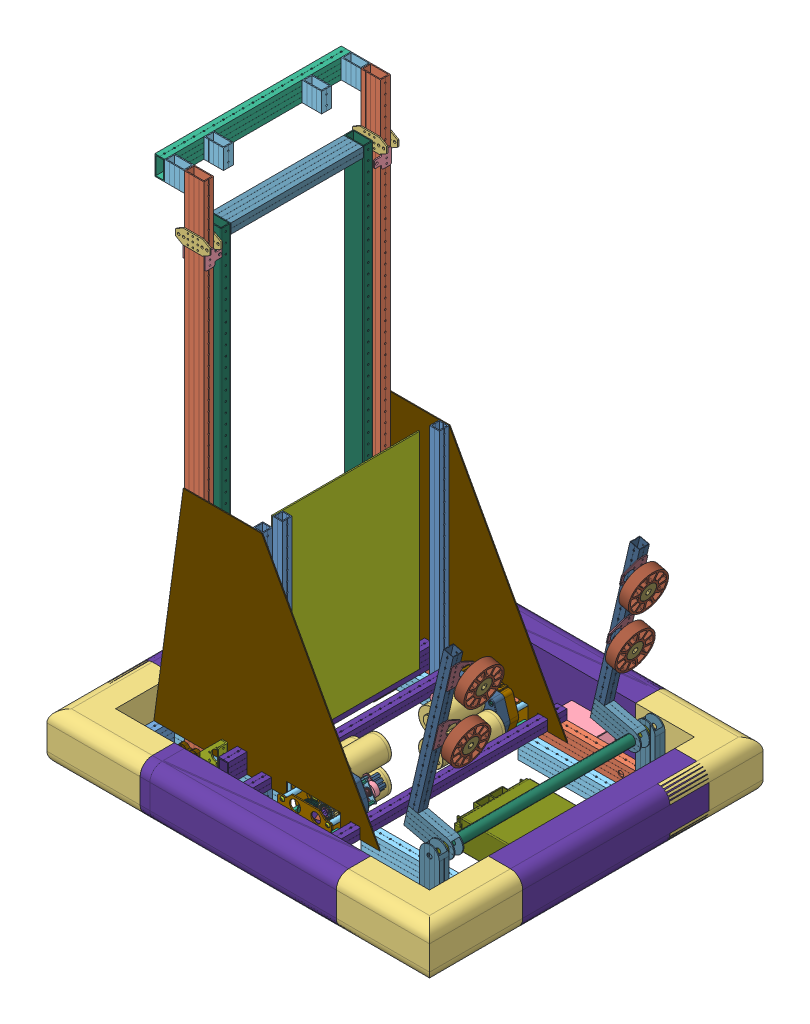
SolidWorks assembly FINAL BOT, configuration Default. Lengths in mm. (continued)
Components (placement in the parent): (continued)
- Elevator Moving Stage-2: Elevator Moving Stage [Default] at (1084.9152 646.5878 79.8495) x (0 0 1) z (-1 0 0) size (444.5 1143 88.9)
  - Elevator Crossbar-1: Elevator Crossbar [Default] at (70.321 -334.7906 927.1918) x (0 1 0) z (1 0 0) size (25.4 50.8 342.9)
  - Elevator Crossbar-2: Elevator Crossbar [Default] at (70.321 738.3594 927.1918) x (0 1 0) z (1 0 0) size (25.4 50.8 342.9)
  - Linear Motion Gusset-2: Linear Motion Gusset [Default] at (479.8486 -372.4027 926.9137) x (0 0 1) z (-1 0 0) size (88.9 73.03 47.09)
    - 217-4399-001 Rev2-1: 217-4399-001 Rev2 [Default] at (0.2781 -0.4879 -0.0474) size (88.9 38.1 3.17)
    - 217-4399-001 Rev2-2: 217-4399-001 Rev2 [Default] at (0.2781 -0.4879 28.5276) size (88.9 38.1 3.17)
    - 217-4399-005 Rev2-1: 217-4399-005 Rev2 [Default] at (25.6781 32.8496 44.0216) x (0 1 0) z (1 0 0) size (41.28 43.91 3.18)
    - 217-4399-005 Rev2-2: 217-4399-005 Rev2 [Default] at (-28.2969 32.8496 44.0216) x (0 1 0) z (1 0 0) size (41.28 43.91 3.18)
  - Elevator Moving Stage Upright-1: Elevator Moving Stage Upright [Default] at (464.021 1.7594 927.1918) x (1 0 0) z (0 1 0) size (25.4 50.8 1143)
  - Elevator Moving Stage Upright-2: Elevator Moving Stage Upright [Default] at (832.321 1.7594 927.1918) x (1 0 0) z (0 1 0) size (25.4 50.8 1143)
  - Linear Motion Gusset-3: Linear Motion Gusset [Default] at (816.4934 -372.4027 927.47) x (0 0 -1) z (1 0 0) size (88.9 73.03 47.09)
    - 217-4399-001 Rev2-1: 217-4399-001 Rev2 [Default] at (0.2781 -0.4879 -0.0474) size (88.9 38.1 3.17)
    - 217-4399-001 Rev2-2: 217-4399-001 Rev2 [Default] at (0.2781 -0.4879 28.5276) size (88.9 38.1 3.17)
    - 217-4399-005 Rev2-1: 217-4399-005 Rev2 [Default] at (25.6781 32.8496 44.0216) x (0 1 0) z (1 0 0) size (41.28 43.91 3.18)
    - 217-4399-005 Rev2-2: 217-4399-005 Rev2 [Default] at (-28.2969 32.8496 44.0216) x (0 1 0) z (1 0 0) size (41.28 43.91 3.18)
  - Custom Elevator Gusset-1: Custom Elevator Gusset [Default] at (425.921 -390.1537 952.5918) size (101.6 127 3.17)
  - Custom Elevator Gusset-2: Custom Elevator Gusset [Default] at (870.421 -390.1537 955.7668) x (-1 0 0) z (0 0 -1) size (101.6 127 3.17)
- Elevator Drive Assembly-1: Elevator Drive Assembly [Default] at (500.2725 546.5466 390.8173) x (-1 0 0) z (0 0 1) size (95.12 72.01 584.2)
  - Elevator Drive Assembly Base Rail-1: Elevator Drive Assembly Base Rail [Default] at (215.5491 266.4994 -119.9968) size (25.4 50.8 584.2)
  - VersaFrame 2 Inch Wide VersaPlanetary Parallel Mount-1: VersaFrame 2 Inch Wide VersaPlanetary Parallel Mount [Default] at (253.5221 266.4359 258.5902) size (73.53 55.5 69.72)
  - 217-2 Stage Versaplanetary STEP-1: 217-2 Stage Versaplanetary STEP [Default] at (253.5221 266.4359 207.0652) x (-1 0 0) z (0 0 -1) size (44.3 44.3 179.1)
    - 217-2625-001 Rev1-1: 217-2625-001 Rev1 [Default] at origin size (42 42 18)
    - 217-2625-002 Rev1-1: 217-2625-002 Rev1 [Default] at (0 0 -29.4) size (42 42 17.13)
    - 217-2625-003 Rev1-1: 217-2625-003 Rev1 [Default] at (0 0 -43.6478) x (1 0 0) z (0 0 -1) size (17 17 64.12)
    - 217-2625-009 Rev1-1: 217-2625-009 Rev1 [Default] at (0 0 -3.48) x (0 -1 0) z (0 0 -1) size (18 18 13)
    - 217-2816-001 Rev1-1: 217-2816-001 Rev1 [Default] at (0 0 -16.85) x (1 0 0) z (0 0 -1) size (42 42 14.5)
    - 217-2625-007 Rev1_Sun_Driver01-1: 217-2625-007 Rev1_Sun_Driver01 [Default] at (0 0 -11.767) x (0.055822 0.998441 0) z (0 0 1) size (14.49 14.49 12.72)
    - 217-2625-100-1: 217-2625-100 [Default] at (0 0 -18.467) x (0 1 0) z (0 0 1) size (39.26 38.9 12.7)
      - 217-2625-008 Rev1-1: 217-2625-008 Rev1 [Default] at origin size (34.7 34.7 4.7)
      - 217-2625-010 Rev1-1: 217-2625-010 Rev1 [Default] at (0 10.193 3.65) x (0.999813 0.019336 0) z (0 0 1) size (4 4 12)
      - 217-2625-010 Rev1-2: 217-2625-010 Rev1 [Default] at (8.691 -5.3258 3.65) size (4 4 12)
      - 217-2625-010 Rev1-3: 217-2625-010 Rev1 [Default] at (-8.691 -5.3258 3.65) size (4 4 12)
      - 217-2625-005 Rev1_Planet_Revolving_Follower01-1: 217-2625-005 Rev1_Planet_Revolving_Follower01 [Default] at (8.691 -5.3258 6.35) x (0.932816 0.360354 0) z (0 0 1) size (16.91 16.92 8)
      - 217-2625-005 Rev1_Planet_Revolving_Follower01-2: 217-2625-005 Rev1_Planet_Revolving_Follower01 [Default] at (-8.691 -5.3258 6.35) x (-0.932788 -0.360426 0) z (0 0 1) size (16.91 16.92 8)
      - 217-2625-005 Rev1_Planet_Revolving_Follower01-3: 217-2625-005 Rev1_Planet_Revolving_Follower01 [Default] at (0 10.193 6.35) x (0.893583 0.448898 0) z (0 0 1) size (16.91 16.92 8)
    - 217-2822-003 Rev4-1: 217-2822-003 Rev4 [Default] at (0 0 9) x (0 1 0) z (0 0 1) size (42 42 4.8)
    - 217-2625-011 Rev1-1: 217-2625-011 Rev1 [Default] at (0 0 1.37) x (1 0 0) z (0 -1 0) size (8.01 7.5 7.94)
    - SSA_SSA0832-0500ZC-1: SSA_SSA0832-0500ZC [Default] at (17.5 -17.5 10.5) x (0.189399 -0.9819 0) z (-0.9819 -0.189399 0) size (6.73 16.76 6.73)
    - 217-2742-1: 217-2742 [Default] at (0 0 -43.1002) x (0 0 1) z (-1 0 0) size (7 28 28)
    - 217-2742-2: 217-2742 [Default] at (0 0 -51.4002) x (0 0 1) z (-0.997393 0.072165 0) size (7 28 28)
    - SSA_SSA0832-1750ZC-1: SSA_SSA0832-1750ZC [Default] at (17.5 -17.5 -47.261) x (1 0 0) z (0 1 0) size (6.73 48.51 6.73)
    - SSA_SSA0832-1750ZC-2: SSA_SSA0832-1750ZC [Default] at (-17.5 17.5 -47.261) x (1 0 0) z (0 1 0) size (6.73 48.51 6.73)
    - 217-2625-018 Rev1_98541A410-1: 217-2625-018 Rev1_98541A410 [Default] at (0 0 -35.4954) x (0 0 -1) z (0.980859 -0.194721 0) size (1 19.6 17.4)
    - 217-2625-017 Rev1_9714K61-1: 217-2625-017 Rev1_9714K61 [Default] at (0 0 -44.1002) x (-0.695225 0.718792 0) z (-0.718792 -0.695225 0) size (28.51 4.98 30.18)
    - PINL-M020-006-S-1: PINL-M020-006-S [Default] at (-18.5 13.6657 -9.5) x (0 0 -1) z (1 0 0) size (6 2 2)
    - PINL-M020-006-S-2: PINL-M020-006-S [Default] at (-18.5 13.6657 -22.2) x (0 0 -1) z (0.23951 -0.970894 0) size (6 2 2)
    - 217-2816-001 Rev1-2: 217-2816-001 Rev1 [Default] at (0 0 -29.55) x (1 0 0) z (0 0 -1) size (42 42 14.5)
    - 217-3106-000 Rev2_NO SUN-1: 217-3106-000 Rev2_NO SUN [Default] at (0 0 -31.5454) size (40.34 37.58 17.71)
      - 217-3106-002 Rev1_Planet_Revolving_Follower01-1: 217-3106-002 Rev1_Planet_Revolving_Follower01 [Default] at (0 10.2965 6.35) x (0.979503 -0.20143 0) z (0 0 1) size (16.8 16.83 8)
      - 217-3106-003 Rev1-1: 217-3106-003 Rev1 [Default] at origin size (34.7 34.7 4.7)
      - 217-3106-001 Rev1_Sun_Driver01-1: 217-3106-001 Rev1_Sun_Driver01 [Default] at (0 0 9.0125) x (1 0 0) z (0 0 -1) size (14.56 14.56 12.7)
      - 217-3106-002 Rev1_Planet_Revolving_Follower01-2: 217-3106-002 Rev1_Planet_Revolving_Follower01 [Default] at (8.917 -5.1482 6.35) x (-0.664195 -0.74756 0) z (0 0 1) size (16.8 16.83 8)
      - 217-3106-002 Rev1_Planet_Revolving_Follower01-3: 217-3106-002 Rev1_Planet_Revolving_Follower01 [Default] at (-8.917 -5.1482 6.35) x (-0.315308 0.948989 0) z (0 0 1) size (16.8 16.83 8)
      - 217-2625-010 Rev1-1: 217-2625-010 Rev1 [Default] at (8.917 -5.1482 3.65) x (0.999617 0.027658 0) z (0 0 1) size (4 4 12)
      - 217-2625-010 Rev1-2: 217-2625-010 Rev1 [Default] at (-8.917 -5.1482 3.65) x (-0.475856 -0.879523 0) z (0 0 1) size (4 4 12)
      - 217-2625-010 Rev1-3: 217-2625-010 Rev1 [Default] at (0 10.2965 3.65) x (-0.523761 0.851865 0) z (0 0 1) size (4 4 12)
    - 775 pro-1: 775 pro [Default] at (0 0 10.5) x (0 0 1) z (-1 0 0) size (88 44.3 44.3)
  - VersaFrame 2 Inch Wide VersaPlanetary Parallel Mount-2: VersaFrame 2 Inch Wide VersaPlanetary Parallel Mount [Default] at (253.5221 266.4359 415.8162) x (1 0 0) z (0 0 -1) size (73.53 55.5 69.72)
  - Hex Shaft Coupler-2: Hex Shaft Coupler [Default] at (253.5221 266.4359 300.4654) x (0.982439 -0.186583 0) z (0 0 -1) size (25.76 22.32 39.56)
    - 217-4008-001 Rev1-1: 217-4008-001 Rev1 [Default] at origin size (25.38 10.66 39.56)
    - 217-4008-001 Rev1-2: 217-4008-001 Rev1 [Default] x (1 0 0) z (0 0 -1) size (25.38 10.66 39.56)
    - 217-4008-002 Rev1_91251A108-1: 217-4008-002 Rev1_91251A108 [Default] at (9.7928 7.025 4.7625) x (0.994016 0 -0.109231) z (0 1 0) size (4.65 4.65 12.51)
    - 217-4008-002 Rev1_91251A108-2: 217-4008-002 Rev1_91251A108 [Default] at (9.7928 7.025 14.2875) x (-0.765668 0 -0.643235) z (0 1 0) size (4.65 4.65 12.51)
    - 217-4008-002 Rev1_91251A108-3: 217-4008-002 Rev1_91251A108 [Default] at (-9.7928 7.025 14.2875) x (-0.114094 0 0.99347) z (0 1 0) size (4.65 4.65 12.51)
    - 217-4008-002 Rev1_91251A108-4: 217-4008-002 Rev1_91251A108 [Default] at (-9.7928 7.025 4.7625) x (0.20346 0 0.979083) z (0 1 0) size (4.65 4.65 12.51)
    - 217-4008-002 Rev1_91251A108-5: 217-4008-002 Rev1_91251A108 [Default] at (-9.7928 -7.025 -4.7625) x (0.20346 0 -0.979083) z (0 -1 0) size (4.65 4.65 12.51)
    - 217-4008-002 Rev1_91251A108-6: 217-4008-002 Rev1_91251A108 [Default] at (-9.7928 -7.025 -14.2875) x (-0.114094 0 -0.99347) z (0 -1 0) size (4.65 4.65 12.51)
    - 217-4008-002 Rev1_91251A108-7: 217-4008-002 Rev1_91251A108 [Default] at (9.7928 -7.025 -14.2875) x (-0.765668 0 0.643235) z (0 -1 0) size (4.65 4.65 12.51)
    - 217-4008-002 Rev1_91251A108-8: 217-4008-002 Rev1_91251A108 [Default] at (9.7928 -7.025 -4.7625) x (0.994016 0 0.109231) z (0 -1 0) size (4.65 4.65 12.51)
  - 12t Aluminum Hub Sprocket (35 Chain, 0.5 Hex Bore)-1: 12t Aluminum Hub Sprocket (35 Chain, 0.5 Hex Bore) [Default] at (253.5221 266.4359 340.2777) x (-0.856405 -0.516304 0) z (0 0 -1) size (40.29 40.29 10.67)
  - 217-2 Stage Versaplanetary STEP-3: 217-2 Stage Versaplanetary STEP [Default] at (253.5221 266.4359 467.3412) size (44.3 44.3 179.1)
    - 217-2625-001 Rev1-1: 217-2625-001 Rev1 [Default] at origin size (42 42 18)
    - 217-2625-002 Rev1-1: 217-2625-002 Rev1 [Default] at (0 0 -29.4) size (42 42 17.13)
    - 217-2625-003 Rev1-1: 217-2625-003 Rev1 [Default] at (0 0 -43.6478) x (1 0 0) z (0 0 -1) size (17 17 64.12)
    - 217-2625-009 Rev1-1: 217-2625-009 Rev1 [Default] at (0 0 -3.48) x (0 -1 0) z (0 0 -1) size (18 18 13)
    - 217-2816-001 Rev1-1: 217-2816-001 Rev1 [Default] at (0 0 -16.85) x (1 0 0) z (0 0 -1) size (42 42 14.5)
    - 217-2625-007 Rev1_Sun_Driver01-1: 217-2625-007 Rev1_Sun_Driver01 [Default] at (0 0 -11.767) x (0.055822 0.998441 0) z (0 0 1) size (14.49 14.49 12.72)
    - 217-2625-100-1: 217-2625-100 [Default] at (0 0 -18.467) x (0 1 0) z (0 0 1) size (39.26 38.9 12.7)
      - 217-2625-008 Rev1-1: 217-2625-008 Rev1 [Default] at origin size (34.7 34.7 4.7)
      - 217-2625-010 Rev1-1: 217-2625-010 Rev1 [Default] at (0 10.193 3.65) x (0.999813 0.019336 0) z (0 0 1) size (4 4 12)
      - 217-2625-010 Rev1-2: 217-2625-010 Rev1 [Default] at (8.691 -5.3258 3.65) size (4 4 12)
      - 217-2625-010 Rev1-3: 217-2625-010 Rev1 [Default] at (-8.691 -5.3258 3.65) size (4 4 12)
      - 217-2625-005 Rev1_Planet_Revolving_Follower01-1: 217-2625-005 Rev1_Planet_Revolving_Follower01 [Default] at (8.691 -5.3258 6.35) x (0.932816 0.360354 0) z (0 0 1) size (16.91 16.92 8)
      - 217-2625-005 Rev1_Planet_Revolving_Follower01-2: 217-2625-005 Rev1_Planet_Revolving_Follower01 [Default] at (-8.691 -5.3258 6.35) x (-0.932788 -0.360426 0) z (0 0 1) size (16.91 16.92 8)
      - 217-2625-005 Rev1_Planet_Revolving_Follower01-3: 217-2625-005 Rev1_Planet_Revolving_Follower01 [Default] at (0 10.193 6.35) x (0.893583 0.448898 0) z (0 0 1) size (16.91 16.92 8)
    - 217-2822-003 Rev4-1: 217-2822-003 Rev4 [Default] at (0 0 9) x (0 1 0) z (0 0 1) size (42 42 4.8)
    - 217-2625-011 Rev1-1: 217-2625-011 Rev1 [Default] at (0 0 1.37) x (1 0 0) z (0 -1 0) size (8.01 7.5 7.94)
    - SSA_SSA0832-0500ZC-1: SSA_SSA0832-0500ZC [Default] at (17.5 -17.5 10.5) x (0.189399 -0.9819 0) z (-0.9819 -0.189399 0) size (6.73 16.76 6.73)
    - 217-2742-1: 217-2742 [Default] at (0 0 -43.1002) x (0 0 1) z (-1 0 0) size (7 28 28)
    - 217-2742-2: 217-2742 [Default] at (0 0 -51.4002) x (0 0 1) z (-0.997393 0.072165 0) size (7 28 28)
    - SSA_SSA0832-1750ZC-1: SSA_SSA0832-1750ZC [Default] at (17.5 -17.5 -47.261) x (1 0 0) z (0 1 0) size (6.73 48.51 6.73)
    - SSA_SSA0832-1750ZC-2: SSA_SSA0832-1750ZC [Default] at (-17.5 17.5 -47.261) x (1 0 0) z (0 1 0) size (6.73 48.51 6.73)
    - 217-2625-018 Rev1_98541A410-1: 217-2625-018 Rev1_98541A410 [Default] at (0 0 -35.4954) x (0 0 -1) z (0.980859 -0.194721 0) size (1 19.6 17.4)
    - 217-2625-017 Rev1_9714K61-1: 217-2625-017 Rev1_9714K61 [Default] at (0 0 -44.1002) x (-0.695225 0.718792 0) z (-0.718792 -0.695225 0) size (28.51 4.98 30.18)
    - PINL-M020-006-S-1: PINL-M020-006-S [Default] at (-18.5 13.6657 -9.5) x (0 0 -1) z (1 0 0) size (6 2 2)
    - PINL-M020-006-S-2: PINL-M020-006-S [Default] at (-18.5 13.6657 -22.2) x (0 0 -1) z (0.23951 -0.970894 0) size (6 2 2)
    - 217-2816-001 Rev1-2: 217-2816-001 Rev1 [Default] at (0 0 -29.55) x (1 0 0) z (0 0 -1) size (42 42 14.5)
    - 217-3106-000 Rev2_NO SUN-1: 217-3106-000 Rev2_NO SUN [Default] at (0 0 -31.5454) size (40.34 37.58 17.71)
      - 217-3106-002 Rev1_Planet_Revolving_Follower01-1: 217-3106-002 Rev1_Planet_Revolving_Follower01 [Default] at (0 10.2965 6.35) x (0.979503 -0.20143 0) z (0 0 1) size (16.8 16.83 8)
      - 217-3106-003 Rev1-1: 217-3106-003 Rev1 [Default] at origin size (34.7 34.7 4.7)
      - 217-3106-001 Rev1_Sun_Driver01-1: 217-3106-001 Rev1_Sun_Driver01 [Default] at (0 0 9.0125) x (1 0 0) z (0 0 -1) size (14.56 14.56 12.7)
      - 217-3106-002 Rev1_Planet_Revolving_Follower01-2: 217-3106-002 Rev1_Planet_Revolving_Follower01 [Default] at (8.917 -5.1482 6.35) x (-0.664195 -0.74756 0) z (0 0 1) size (16.8 16.83 8)
      - 217-3106-002 Rev1_Planet_Revolving_Follower01-3: 217-3106-002 Rev1_Planet_Revolving_Follower01 [Default] at (-8.917 -5.1482 6.35) x (-0.315308 0.948989 0) z (0 0 1) size (16.8 16.83 8)
      - 217-2625-010 Rev1-1: 217-2625-010 Rev1 [Default] at (8.917 -5.1482 3.65) x (0.999617 0.027658 0) z (0 0 1) size (4 4 12)
      - 217-2625-010 Rev1-2: 217-2625-010 Rev1 [Default] at (-8.917 -5.1482 3.65) x (-0.475856 -0.879523 0) z (0 0 1) size (4 4 12)
      - 217-2625-010 Rev1-3: 217-2625-010 Rev1 [Default] at (0 10.2965 3.65) x (-0.523761 0.851865 0) z (0 0 1) size (4 4 12)
    - 775 pro-1: 775 pro [Default] at (0 0 10.5) x (0 0 1) z (-1 0 0) size (88 44.3 44.3)
  - Hex Shaft Coupler-3: Hex Shaft Coupler [Default] at (253.5221 266.4359 373.941) x (0.576903 -0.816813 0) z (0 0 -1) size (25.76 22.32 39.56)
    - 217-4008-001 Rev1-1: 217-4008-001 Rev1 [Default] at origin size (25.38 10.66 39.56)
    - 217-4008-001 Rev1-2: 217-4008-001 Rev1 [Default] x (1 0 0) z (0 0 -1) size (25.38 10.66 39.56)
    - 217-4008-002 Rev1_91251A108-1: 217-4008-002 Rev1_91251A108 [Default] at (9.7928 7.025 4.7625) x (0.994016 0 -0.109231) z (0 1 0) size (4.65 4.65 12.51)
    - 217-4008-002 Rev1_91251A108-2: 217-4008-002 Rev1_91251A108 [Default] at (9.7928 7.025 14.2875) x (-0.765668 0 -0.643235) z (0 1 0) size (4.65 4.65 12.51)
    - 217-4008-002 Rev1_91251A108-3: 217-4008-002 Rev1_91251A108 [Default] at (-9.7928 7.025 14.2875) x (-0.114094 0 0.99347) z (0 1 0) size (4.65 4.65 12.51)
    - 217-4008-002 Rev1_91251A108-4: 217-4008-002 Rev1_91251A108 [Default] at (-9.7928 7.025 4.7625) x (0.20346 0 0.979083) z (0 1 0) size (4.65 4.65 12.51)
    - 217-4008-002 Rev1_91251A108-5: 217-4008-002 Rev1_91251A108 [Default] at (-9.7928 -7.025 -4.7625) x (0.20346 0 -0.979083) z (0 -1 0) size (4.65 4.65 12.51)
    - 217-4008-002 Rev1_91251A108-6: 217-4008-002 Rev1_91251A108 [Default] at (-9.7928 -7.025 -14.2875) x (-0.114094 0 -0.99347) z (0 -1 0) size (4.65 4.65 12.51)
    - 217-4008-002 Rev1_91251A108-7: 217-4008-002 Rev1_91251A108 [Default] at (9.7928 -7.025 -14.2875) x (-0.765668 0 0.643235) z (0 -1 0) size (4.65 4.65 12.51)
    - 217-4008-002 Rev1_91251A108-8: 217-4008-002 Rev1_91251A108 [Default] at (9.7928 -7.025 -4.7625) x (0.994016 0 0.109231) z (0 -1 0) size (4.65 4.65 12.51)
  - VersaFrame Corner Gusset-1: VersaFrame Corner Gusset [Default] at (228.2491 291.8994 603.9032) x (0 -1 0) z (0 0 1) size (69.72 69.72 25.4)
  - VersaFrame Corner Gusset-2: VersaFrame Corner Gusset [Default] at (228.2491 291.8994 70.5032) x (1 0 0) z (0 0 -1) size (69.72 69.72 25.4)
- Elevator Bottom Shaft-1: Elevator Bottom Shaft [Default] at (109.0247 229.2599 486.7205) size (14.48 12.67 431.8)
- VersaFrame Face Bearing Mount-1: VersaFrame Face Bearing Mount [Default] at (132.1964 229.3742 537.5205) size (101.35 50.55 2.29)
- Intake Mechanism-1: Intake Mechanism [Default] at (970.1621 668.6497 267.2449) x (-0.974229 0.225563 0) z (0 0 1) size (127 459.2 565.18)
  - Intake Arm-1: Intake Arm [Default] at (166.6282 -436.1132 702.0756) x (0 0 1) z (0 1 0) size (25.4 25.4 406.4)
  - am-3480+4IN+500Hex+Bore+Compliant+Wheel-1: am-3480+4IN+500Hex+Bore+Compliant+Wheel [Default] at (107.5902 -52.3006 677.3515) x (0 -1 0) z (1 0 0) size (101.6 101.6 25.74)
    - 4IN Compliant Wheel FINAL Overmold-1: 4IN Compliant Wheel FINAL Overmold [Default] at (-16.2374 3.8509 18.652) size (101.6 101.6 25.74)
    - 2in Wheel Intergrated 0500 HEX Hub-1: 2in Wheel Intergrated 0500 HEX Hub [Default] at (-16.2374 3.8509 5.952) x (-1 0 0) z (0 0 -1) size (41.91 41.91 25.4)
  - VersaFrame Side Bearing Mount-1: VersaFrame Side Bearing Mount [Default] at (151.6422 -36.0632 673.5006) x (0 1 0) z (1 0 0) size (63.5 61.91 2.29)
  - am-3480+4IN+500Hex+Bore+Compliant+Wheel-2: am-3480+4IN+500Hex+Bore+Compliant+Wheel [Default] at (107.5902 102.0213 664.9245) x (0 -0.716102 -0.697996) z (1 0 0) size (101.6 101.6 25.74)
    - 4IN Compliant Wheel FINAL Overmold-1: 4IN Compliant Wheel FINAL Overmold [Default] at (-16.2374 3.8509 18.652) size (101.6 101.6 25.74)
    - 2in Wheel Intergrated 0500 HEX Hub-1: 2in Wheel Intergrated 0500 HEX Hub [Default] at (-16.2374 3.8509 5.952) x (-1 0 0) z (0 0 -1) size (41.91 41.91 25.4)
  - VersaFrame Side Bearing Mount-2: VersaFrame Side Bearing Mount [Default] at (151.6422 116.3368 673.5006) x (0 1 0) z (1 0 0) size (63.5 61.91 2.29)
  - VersaFrame Side Bearing Mount-3: VersaFrame Side Bearing Mount [Default] at (151.6422 -36.0632 248.0506) x (0 -1 0) z (1 0 0) size (63.5 61.91 2.29)
  - am-3480+4IN+500Hex+Bore+Compliant+Wheel-3: am-3480+4IN+500Hex+Bore+Compliant+Wheel [Default] at (107.5902 103.4135 258.6086) x (0 -0.899512 0.436896) z (1 0 0) size (101.6 101.6 25.74)
    - 4IN Compliant Wheel FINAL Overmold-1: 4IN Compliant Wheel FINAL Overmold [Default] at (-16.2374 3.8509 18.652) size (101.6 101.6 25.74)
    - 2in Wheel Intergrated 0500 HEX Hub-1: 2in Wheel Intergrated 0500 HEX Hub [Default] at (-16.2374 3.8509 5.952) x (-1 0 0) z (0 0 -1) size (41.91 41.91 25.4)
  - VersaFrame Side Bearing Mount-4: VersaFrame Side Bearing Mount [Default] at (151.6422 116.3368 248.0506) x (0 -1 0) z (1 0 0) size (63.5 61.91 2.29)
  - am-3480+4IN+500Hex+Bore+Compliant+Wheel-4: am-3480+4IN+500Hex+Bore+Compliant+Wheel [Default] at (107.5902 -19.397 247.2002) x (0 0.983506 0.180877) z (1 0 0) size (101.6 101.6 25.74)
    - 4IN Compliant Wheel FINAL Overmold-1: 4IN Compliant Wheel FINAL Overmold [Default] at (-16.2374 3.8509 18.652) size (101.6 101.6 25.74)
    - 2in Wheel Intergrated 0500 HEX Hub-1: 2in Wheel Intergrated 0500 HEX Hub [Default] at (-16.2374 3.8509 5.952) x (-1 0 0) z (0 0 -1) size (41.91 41.91 25.4)
  - Intake Arm-2: Intake Arm [Default] at (166.6282 -436.1132 219.4756) x (0 0 1) z (0 1 0) size (25.4 25.4 406.4)
  - Intake Upright 2-1: Intake Upright 2 [Default] at (801.6282 338.5868 219.4756) x (0 0 1) z (-1 0 0) size (25.4 50.8 127)
  - Intake Upright 2-2: Intake Upright 2 [Default] at (801.6282 338.5868 702.0756) x (0 0 1) z (-1 0 0) size (25.4 50.8 127)
  - Intake Round Crossbar-1: Intake Round Crossbar [Default] at (77.7282 338.663 232.1756) size (25.4 25.4 457.2)
- Intake Upright 2-1: Intake Upright 2 [Default] at (818.1234 -367.6528 448.6205) x (0 0 -1) z (0 1 0) size (25.4 50.8 127)
- Intake Upright 2-3: Intake Upright 2 [Default] at (818.1234 -367.6528 1007.4205) x (0 0 -1) z (0 1 0) size (25.4 50.8 127)
- Intake Round Crossbar .5 depth-1: Intake Round Crossbar .5 depth [Default] at (818.0472 356.2472 16.8205) size (25.4 25.4 12.7)
- Intake Round Crossbar .5 depth-2: Intake Round Crossbar .5 depth [Default] at (818.0472 356.2472 537.5205) size (25.4 25.4 12.7)
- Blue Bumper Side-1: Blue Bumper Side [Default] at (233.9234 330.8472 296.2205) x (1 0 0) z (0 0 -1) size (482.6 127 88.9)
- Blue Bumper-1: Blue Bumper [Default] at (-32.7766 203.8472 296.2205) x (0 0 1) z (-1 0 0) size (241.3 127 241.3)
- Electronics Upright-1: Electronics Upright [Default] at (322.8234 64.1472 956.6205) x (-1 0 0) z (0 1 0) size (25.4 25.4 609.6)
- Electronics Upright-2: Electronics Upright [Default] at (322.8234 64.1472 499.4205) x (-1 0 0) z (0 1 0) size (25.4 25.4 609.6)
- Side support Panal-1: Side support Panal [Default] at (489.9994 334.5018 486.7205) x (-1 0 0) z (0 0 -1) size (584.2 558.8 2.54)
- Side support Panal-2: Side support Panal [Default] at (489.9994 334.5018 971.8605) x (-1 0 0) z (0 0 -1) size (584.2 558.8 2.54)
- Blue Bumper Side-2: Blue Bumper Side [Default] at (957.8234 330.8472 435.9205) x (0 0 1) z (1 0 0) size (482.6 127 88.9)
- Blue Bumper Side-4: Blue Bumper Side [Default] at (716.5234 330.8472 1159.8205) x (-1 0 0) z (0 0 1) size (482.6 127 88.9)
- Blue Bumper Side-5: Blue Bumper Side [Default] at (208.5234 330.8472 296.2205) x (1 0 0) z (0 0 -1) size (482.6 127 88.9)
- Blue Bumper Side-6: Blue Bumper Side [Default] at (-32.7766 330.8472 1020.1205) x (0 0 -1) z (-1 0 0) size (482.6 127 88.9)
- Blue Bumper Side-7: Blue Bumper Side [Default] at (691.1234 330.8472 1159.8205) x (-1 0 0) z (0 0 1) size (482.6 127 88.9)
- Blue Bumper-3: Blue Bumper [Default] at (-32.7766 330.8472 1159.8205) x (0 0 -1) z (-1 0 0) size (241.3 127 241.3)
Mates (geometry in assembly coordinates):
- Coincident2: coincident aligned: plane of Test Base 3-1/Base Side Rail Internal-1 through (360.9234 203.8472 943.9205) normal (0 -1 0); plane of Elevator Base Frame-1/Elevator Fixed Frame-1 through (157.7234 203.8472 956.6205) normal (0 -1 0)
- Distance1: distance = 50.8 mm anti-aligned: plane of Elevator Base Frame-1/Elevator Fixed Frame-1 through (132.3234 1524.6472 943.9205) normal (-1 0 0); plane of Test Base 3-1/Base Rear Rail-1 through (81.5234 203.8472 1070.9205) normal (1 0 0)
- Coincident4: coincident anti-aligned: plane of Elevator Base Frame-1/Elevator Fixed Frame-1 through (132.3234 1524.6472 969.3205) normal (0 0 1); plane of ? through (132.3234 254.6472 969.3205) normal (0 0 -1)
- Coincident5: coincident aligned: plane of Elevator Base Frame-1/Elevator Fixed Frame-1 through (132.3234 1524.6472 943.9205) normal (-1 0 0); plane of ? through (132.3234 254.6472 972.4955) normal (-1 0 0)
- Coincident7: coincident anti-aligned: plane of Elevator Base Frame-1/Elevator Fixed Frame-2 through (132.3234 1524.6472 486.7205) normal (0 0 -1); plane of ? through (132.3234 254.6472 486.7205) normal (0 0 1)
- Coincident9: coincident aligned: plane of Elevator Base Frame-1/Elevator Fixed Frame-2 through (132.3234 1524.6472 486.7205) normal (-1 0 0); plane of ? through (132.3234 254.6472 486.7205) normal (-1 0 0)
- Coincident10: coincident anti-aligned: plane of Test Base 3-1/Base Side Rail Internal-1 through (360.9234 254.6472 943.9205) normal (0 1 0); plane of ? through (132.3234 254.6472 972.4955) normal (0 -1 0)
- Coincident11: coincident anti-aligned: plane of Test Base 3-1/Base Side Rail Internal-4 through (81.5234 254.6472 512.1205) normal (0 1 0); plane of ? through (132.3234 254.6472 486.7205) normal (0 -1 0)
- Coincident13: coincident aligned: plane of Test Base 3-1/Electronics Upright-1 through (322.8234 813.4472 905.8205) normal (0 1 0); plane of Electronics Panel-1 through (310.1234 813.4472 918.5205) normal (0 1 0)
- Coincident14: coincident anti-aligned: plane of ? through (132.3234 254.6472 969.3205) normal (0 0 -1); plane of Electronics Panel-1 through (310.1234 280.0472 969.3205) normal (0 0 1)
- Coincident20: coincident anti-aligned: plane of Test Base 3-1/Electronics Upright-2 through (310.1234 203.8472 537.5205) normal (-1 0 0); plane of Electronics Panel-1 through (310.1234 280.0472 918.5205) normal (1 0 0)
- Coincident46: coincident aligned: plane of Test Base 3-1/Base Rear Rail-1 through (56.1234 203.8472 1070.9205) normal (0 -1 0); plane of Elevator Base Frame-1/Elevator Fixed Frame-1 through (157.7234 203.8472 956.6205) normal (0 -1 0)
- Coincident57: coincident anti-aligned: plane of Test Base 3-1/Base Side Rail Internal-1 through (360.9234 203.8472 943.9205) normal (0 0 1); plane of Elevator Base Frame-1/Elevator Fixed Frame-1 through (132.3234 1524.6472 943.9205) normal (0 0 -1)
- Concentric9: concentric anti-aligned: circle of Test Base 3-1/Base Side Rail-2; cylinder of 6 inch Traction Wheel and Tire-1/6 inch Traction Wheel-1/217-2589-001 Rev3-1 through (170.4234 229.171 400.9955) axis (0 0 1) radius 14.3
- Distance26: distance = 12.7 mm aligned: plane of Test Base 3-1/Base Side Rail-2 through (81.5234 203.8472 435.9205) normal (0 0 -1); plane of 6 inch Traction Wheel and Tire-1/6 inch Traction Wheel-1/217-2589-001 Rev3-2 through (170.4234 229.171 423.2205) normal (0 0 -1)
- Distance27: distance = 19.05 mm anti-aligned: plane of Elevator Moving Stage-2/Elevator Moving Stage Upright-1 through (134.8634 1397.6472 531.1705) normal (0 0 -1); plane of Elevator Base Frame-1/Elevator Fixed Frame-2 through (132.3234 1524.6472 512.1205) normal (0 0 1)
- Coincident58: coincident aligned: plane of Elevator Base Frame-1/Elevator Fixed Frame-2 through (132.3234 1524.6472 486.7205) normal (-1 0 0); plane of Elevator Moving Stage-2/Elevator Moving Stage Upright-1 through (132.3234 1397.6472 533.7105) normal (-1 0 0)
- LimitDistance2: limit distance = -127 mm aligned: plane of Elevator Moving Stage-2/Elevator Crossbar-2 through (157.7234 1397.6472 150.1705) normal (0 1 0); plane of Elevator Base Frame-1/Elevator Fixed Frame-1 through (157.7234 1524.6472 956.6205) normal (0 1 0)
- Coincident60: coincident aligned: plane of Test Base 3-1/Base Side Rail-1 through (81.5234 203.8472 1020.1205) normal (0 0 1); plane of Elevator Drive Assembly-1/Elevator Drive Assembly Base Rail-1 through (284.7234 280.0472 1020.1205) normal (0 0 1)
- Coincident61: coincident anti-aligned: plane of Test Base 3-1/Base Side Rail Internal-4 through (81.5234 203.8472 537.5205) normal (0 0 1); plane of VersaFrame Face Bearing Mount-1 through (81.5234 204.1012 537.5205) normal (0 0 -1)
- Coincident62: coincident aligned: plane of Test Base 3-1/Base Side Rail Internal-4 through (81.5234 254.6472 512.1205) normal (0 1 0); plane of VersaFrame Face Bearing Mount-1 through (81.5234 254.6472 539.8065) normal (0 1 0)
- Coincident63: coincident anti-aligned: plane of Test Base 3-1/Base Rear Rail-1 through (81.5234 203.8472 1070.9205) normal (1 0 0); plane of VersaFrame Face Bearing Mount-1 through (81.5234 254.6472 539.8065) normal (-1 0 0)
- Coincident64: coincident aligned: plane of Test Base 3-1/Base Side Rail Internal-4 through (81.5234 203.8472 512.1205) normal (0 0 -1); plane of Elevator Bottom Shaft-1 through (109.0247 229.2599 512.1205) normal (0 0 -1)
- Distance29: distance = 19.05 mm aligned: plane of Elevator Bottom Shaft-1 through (112.6835 235.5972 943.9205) normal (0 1 0); plane of Test Base 3-1/Base Rear Rail-1 through (56.1234 254.6472 1070.9205) normal (0 1 0)
- Coincident65: coincident anti-aligned: plane of Test Base 3-1/Base Side Rail Internal-1 through (360.9234 254.6472 943.9205) normal (0 1 0); plane of Elevator Drive Assembly-1/Elevator Drive Assembly Base Rail-1 through (297.4234 254.6472 1020.1205) normal (0 -1 0)
- Distance30: distance = 88.9 mm anti-aligned: plane of Elevator Drive Assembly-1/Elevator Drive Assembly Base Rail-1 through (272.0234 305.4472 1020.1205) normal (-1 0 0); plane of Elevator Base Frame-1/Elevator Fixed Frame-1 through (183.1234 1524.6472 943.9205) normal (1 0 0)
- Coincident66: coincident: line of Test Base 3-1/Base Side Rail-2 through (777.9547 254.6472 448.5443) axis (-1 0 0); plane of Intake Upright 2-1 through (818.1234 254.6472 448.6205) normal (0 -1 0)
- Coincident67: coincident aligned: plane of Test Base 3-1/Base Side Rail-2 through (81.5234 203.8472 435.9205) normal (0 0 -1); plane of Intake Upright 2-1 through (818.1234 -367.6528 435.9205) normal (0 0 -1)
- Coincident68: coincident anti-aligned: plane of Test Base 3-1/Base Front Rail-2 through (843.5234 203.8472 537.5205) normal (-1 0 0); plane of Intake Upright 2-1 through (843.5234 381.6472 461.3205) normal (1 0 0)
- Concentric10: concentric anti-aligned: cylinder of Intake Mechanism-1/Intake Upright 2-1 through (818.0472 356.2472 474.0205) axis (0 0 1) radius 6.35; cylinder of Intake Upright 2-1 through (818.0472 356.2472 461.3205) axis (0 0 -1) radius 6.35
- Parallel1: parallel aligned: plane of Test Base 3-1/Base Side Rail Internal-5 through (843.5234 203.8472 512.1205) normal (0 0 -1); plane of Intake Mechanism-1/Intake Upright 2-1 through (112.8203 519.6066 474.0205) normal (0 0 -1)
- Coincident70: coincident anti-aligned: plane of Test Base 3-1/Base Side Rail-1 through (81.5234 254.6472 994.7205) normal (0 1 0); plane of Intake Upright 2-3 through (818.1234 254.6472 1007.4205) normal (0 -1 0)
- Coincident71: coincident aligned: plane of Test Base 3-1/Base Side Rail-1 through (81.5234 203.8472 1020.1205) normal (0 0 1); plane of Intake Upright 2-3 through (818.1234 -367.6528 1020.1205) normal (0 0 1)
- Coincident72: coincident anti-aligned: plane of Test Base 3-1/Base Front Rail-1 through (843.5234 203.8472 1070.9205) normal (-1 0 0); plane of Intake Upright 2-3 through (843.5234 381.6472 1020.1205) normal (1 0 0)
- Concentric11: concentric anti-aligned: cylinder of Intake Mechanism-1/Intake Upright 2-1 through (818.0472 356.2472 474.0205) axis (0 0 1) radius 6.35; cylinder of Intake Upright 2-1 through (818.0472 356.2472 461.3205) axis (0 0 -1) radius 6.35
- Concentric12: concentric anti-aligned: cylinder of Intake Mechanism-1/Intake Upright 2-2 through (818.0472 356.2472 956.6205) axis (0 0 1) radius 6.35; cylinder of Intake Upright 2-3 through (818.0472 356.2472 1020.1205) axis (0 0 -1) radius 6.35
- Coincident73: coincident anti-aligned: plane of Intake Upright 2-3 through (818.1234 -367.6528 994.7205) normal (0 0 -1); plane of Intake Round Crossbar .5 depth-2 through (818.0472 356.2472 994.7205) normal (0 0 1)
- Concentric13: concentric aligned: cylinder of Intake Upright 2-3 through (818.0472 356.2472 1020.1205) axis (0 0 -1) radius 6.35; cylinder of Intake Round Crossbar .5 depth-2 through (818.0472 356.2472 994.7205) axis (0 0 -1) radius 11.1125
- Coincident74: coincident anti-aligned: plane of Intake Mechanism-1/Intake Upright 2-2 through (112.8203 519.6066 982.0205) normal (0 0 1); plane of Intake Round Crossbar .5 depth-2 through (694.3591 381.6472 982.0205) normal (0 0 -1)
- Coincident75: coincident anti-aligned: plane of Intake Upright 2-1 through (818.1234 -367.6528 461.3205) normal (0 0 1); plane of Intake Round Crossbar .5 depth-1 through (694.3591 381.6472 461.3205) normal (0 0 -1)
- Concentric14: concentric aligned: cylinder of Intake Upright 2-1 through (818.0472 356.2472 461.3205) axis (0 0 -1) radius 6.35; cylinder of Intake Round Crossbar .5 depth-1 through (818.0472 356.2472 474.0205) axis (0 0 -1) radius 11.1125
- Coincident76: coincident aligned: plane of Test Base 3-1/Blue Bumper-2 through (957.8234 330.8472 385.1205) normal (0 0 1); plane of Blue Bumper Side-1 through (716.5234 330.8472 385.1205) normal (0 0 1)
- Coincident77: coincident anti-aligned: plane of Test Base 3-1/Blue Bumper-2 through (716.5234 330.8472 296.2205) normal (-1 0 0); plane of Blue Bumper Side-1 through (716.5234 330.8472 296.2205) normal (1 0 0)
- Coincident78: coincident aligned: plane of Test Base 3-1/Blue Bumper-2 through (957.8234 203.8472 296.2205) normal (0 -1 0); plane of Blue Bumper Side-1 through (716.5234 203.8472 296.2205) normal (0 -1 0)
- Coincident79: coincident anti-aligned: plane of Blue Bumper Side-1 through (233.9234 330.8472 296.2205) normal (-1 0 0); plane of ?
- Coincident80: coincident aligned: plane of Blue Bumper Side-1 through (716.5234 330.8472 296.2205) normal (0 1 0); plane of ?
- Coincident81: coincident aligned: plane of Test Base 3-1/Electronics Upright-1 through (310.1234 203.8472 918.5205) normal (0 0 1); plane of Electronics Panel-1 through (310.1234 280.0472 918.5205) normal (0 0 1)
- Coincident84: coincident anti-aligned: plane of Test Base 3-1/Base Side Rail Internal-1 through (360.9234 203.8472 943.9205) normal (0 0 1); plane of Electronics Upright-1 through (335.5234 813.4472 943.9205) normal (0 0 -1)
- Coincident86: coincident aligned: plane of Test Base 3-1/Base Side Rail Internal-1 through (360.9234 203.8472 943.9205) normal (0 -1 0); plane of Electronics Upright-1 through (322.8234 203.8472 956.6205) normal (0 -1 0)
- Coincident88: coincident: line of Test Base 3-1/Base Side Rail Internal-4 through (360.9234 254.6472 512.1205) axis (-1 0 0); plane of Electronics Upright-2 through (335.5234 813.4472 512.1205) normal (0 0 1)
- Coincident89: coincident aligned: plane of Test Base 3-1/Base Side Rail Internal-4 through (81.5234 203.8472 512.1205) normal (0 -1 0); plane of Electronics Upright-2 through (322.8234 203.8472 499.4205) normal (0 -1 0)
- Coincident90: coincident: line of Elevator Base Frame-1/Elevator Fixed Frame-2 through (157.6472 203.8472 486.7205) axis (0 1 0); plane of Side support Panal-1 through (489.9994 334.5018 486.7205) normal (0 0 1)
- Coincident91: coincident anti-aligned: plane of Elevator Drive Assembly-1/Elevator Drive Assembly Base Rail-1 through (297.4234 305.4472 1020.1205) normal (1 0 0); plane of Side support Panal-1 through (297.4234 334.5018 484.1805) normal (-1 0 0)
- Coincident92: coincident anti-aligned: plane of Test Base 3-1/Base Rear Rail-1 through (56.1234 254.6472 1070.9205) normal (0 1 0); plane of Side support Panal-1 through (489.9994 254.6472 484.1805) normal (0 -1 0)
- Coincident93: coincident anti-aligned: plane of Test Base 3-1/Superstructure Lower Crossbar-2 through (335.5234 254.6472 435.9205) normal (-1 0 0); plane of Electronics Upright-2 through (335.5234 813.4472 486.7205) normal (1 0 0)
- Coincident94: coincident anti-aligned: plane of Test Base 3-1/Superstructure Lower Crossbar-2 through (335.5234 254.6472 435.9205) normal (-1 0 0); plane of Electronics Upright-1 through (335.5234 813.4472 943.9205) normal (1 0 0)
- Coincident95: coincident anti-aligned: plane of Elevator Base Frame-1/Elevator Fixed Frame-1 through (132.3234 1524.6472 969.3205) normal (0 0 1); plane of Side support Panal-2 through (489.9994 334.5018 969.3205) normal (0 0 -1)
- Coincident96: coincident aligned: line of Test Base 3-1/Base Rear Rail-1 through (56.1234 254.6472 385.1205) axis (0 0 1); line of Side support Panal-2 through (56.1234 254.6472 969.3205) axis (0 0 1)
- Coincident97: coincident anti-aligned: plane of Elevator Drive Assembly-1/Elevator Drive Assembly Base Rail-1 through (297.4234 305.4472 1020.1205) normal (0 1 0); plane of Side support Panal-2 through (489.9994 305.4472 969.3205) normal (0 -1 0)
- Coincident98: coincident anti-aligned: plane of Test Base 3-1/Blue Bumper-1 through (957.8234 330.8472 918.5205) normal (0 0 -1); plane of Blue Bumper Side-2 through (957.8234 330.8472 918.5205) normal (0 0 1)
- Coincident99: coincident aligned: plane of Test Base 3-1/Blue Bumper-1 through (957.8234 203.8472 1159.8205) normal (0 -1 0); plane of Blue Bumper Side-2 through (957.8234 203.8472 918.5205) normal (0 -1 0)
- Coincident100: coincident aligned: plane of Test Base 3-1/Blue Bumper-1 through (957.8234 330.8472 1159.8205) normal (1 0 0); plane of Blue Bumper Side-2 through (957.8234 330.8472 918.5205) normal (1 0 0)
- Coincident101: coincident anti-aligned: plane of Test Base 3-1/Base Rear Rail-1 through (56.1234 203.8472 1070.9205) normal (-1 0 0); plane of Blue Bumper-1 through (56.1234 330.8472 296.2205) normal (1 0 0)
- Coincident102: coincident anti-aligned: plane of Test Base 3-1/Base Rear Rail-1 through (68.8234 229.2472 385.1205) normal (0 0 -1); plane of Blue Bumper-1 through (-32.7766 330.8472 385.1205) normal (0 0 1)
- Coincident103: coincident aligned: plane of Blue Bumper Side-1 through (716.5234 203.8472 296.2205) normal (0 -1 0); plane of Blue Bumper-1 through (-32.7766 203.8472 296.2205) normal (0 -1 0)
- Coincident104: coincident aligned: plane of Test Base 3-1/Blue Bumper-1 through (716.5234 330.8472 1159.8205) normal (-1 0 0); plane of ? through (716.5234 248.8661 1038.1024) normal (-1 0 0)
- Coincident105: coincident anti-aligned: plane of Test Base 3-1/Blue Bumper-1 through (716.5234 330.8472 1159.8205) normal (-1 0 0); plane of Blue Bumper Side-4 through (716.5234 330.8472 1159.8205) normal (1 0 0)
- Coincident106: coincident aligned: plane of Test Base 3-1/Blue Bumper-1 through (957.8234 330.8472 1159.8205) normal (0 0 1); plane of Blue Bumper Side-4 through (233.9234 330.8472 1159.8205) normal (0 0 1)
- Coincident107: coincident aligned: plane of Test Base 3-1/Blue Bumper-1 through (957.8234 330.8472 1159.8205) normal (0 1 0); plane of Blue Bumper Side-4 through (233.9234 330.8472 1159.8205) normal (0 1 0)
- Coincident108: coincident anti-aligned: plane of Blue Bumper-1 through (208.5234 330.8472 296.2205) normal (1 0 0); plane of Blue Bumper Side-5 through (208.5234 330.8472 296.2205) normal (-1 0 0)
- Coincident109: coincident aligned: plane of Blue Bumper-1 through (-32.7766 330.8472 296.2205) normal (0 1 0); plane of Blue Bumper Side-5 through (691.1234 330.8472 296.2205) normal (0 1 0)
- Coincident110: coincident aligned: plane of Blue Bumper-1 through (-32.7766 330.8472 296.2205) normal (0 0 -1); plane of Blue Bumper Side-5 through (691.1234 330.8472 296.2205) normal (0 0 -1)
- Coincident111: coincident anti-aligned: plane of Blue Bumper-1 through (-32.7766 330.8472 537.5205) normal (0 0 1); plane of Blue Bumper Side-6 through (-32.7766 330.8472 537.5205) normal (0 0 -1)
- Coincident112: coincident aligned: plane of Blue Bumper-1 through (-32.7766 330.8472 296.2205) normal (-1 0 0); plane of Blue Bumper Side-6 through (-32.7766 330.8472 537.5205) normal (-1 0 0)
- Coincident113: coincident aligned: plane of Blue Bumper-1 through (-32.7766 330.8472 296.2205) normal (0 1 0); plane of Blue Bumper Side-6 through (-32.7766 330.8472 537.5205) normal (0 1 0)
- Coincident115: coincident: line of Test Base 3-1/Base Rear Rail-1 through (56.1234 242.0234 1070.9205) axis (0 0 -1); plane of Blue Bumper-3 through (56.1234 203.8472 1159.8205) normal (1 0 0)
- Coincident116: coincident anti-aligned: plane of Test Base 3-1/Base Rear Rail-1 through (68.8234 229.2472 1070.9205) normal (0 0 1); plane of Blue Bumper-3 through (-32.7766 203.8472 1070.9205) normal (0 0 -1)
- Coincident117: coincident aligned: plane of Blue Bumper Side-6 through (-32.7766 330.8472 537.5205) normal (0 1 0); plane of Blue Bumper-3 through (-32.7766 330.8472 1159.8205) normal (0 1 0)
- Coincident118: coincident aligned: plane of Blue Bumper Side-4 through (233.9234 203.8472 1159.8205) normal (0 -1 0); plane of Blue Bumper Side-7 through (208.5234 203.8472 1159.8205) normal (0 -1 0)
- Coincident119: coincident anti-aligned: plane of Blue Bumper Side-7 through (208.5234 330.8472 1159.8205) normal (-1 0 0); plane of Blue Bumper-3 through (208.5234 203.8472 1159.8205) normal (1 0 0)
- Coincident120: coincident aligned: plane of Blue Bumper Side-7 through (208.5234 203.8472 1159.8205) normal (0 -1 0); plane of Blue Bumper-3 through (-32.7766 203.8472 1159.8205) normal (0 -1 0)
- Coincident121: coincident aligned: plane of Blue Bumper Side-7 through (208.5234 330.8472 1070.9205) normal (0 0 -1); plane of Blue Bumper-3 through (-32.7766 203.8472 1070.9205) normal (0 0 -1)
